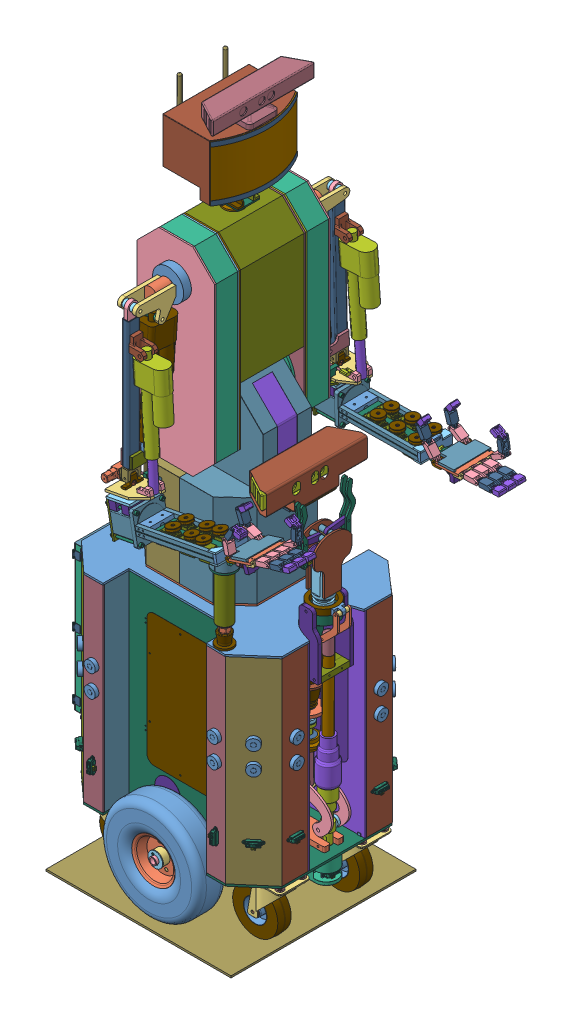
SolidWorks assembly sorbot, configuration По умолчанию. Lengths in mm. (continued)
Mates (geometry in assembly coordinates): (continued)
- Расстояние24: distance = 14 mm anti-aligned: plane of ? through (171.0986 905.6533 109.8374) normal (0.9762 0.216874 0); plane of ? through (184.7654 908.6895 127.5946) normal (-0.9762 -0.216874 0)
- Заблокировать539: lock: unknown of lower.arm.p2-1; unknown of arm.rotate.p9-1
- Заблокировать540: lock: unknown of lower.arm.p2-3; unknown of arm.rotate.p9-1
- Расстояние25: distance = 0.5 mm anti-aligned: plane of lower.arm.p3-1 through (42.4949 859.0482 146.4722) normal (-0.982605 -0.185706 0); plane of arm.rotate-1/SY85STH65-2808A-1 through (42.1893 857.9727 140.2746) normal (0.982605 0.185706 0)
- Заблокировать541: lock: unknown of lower.arm.p2-2; unknown of arm.rotate.p9-2
- Совпадение1112: coincident anti-aligned: plane of lower.arm.p3-1 through (42.4949 859.0482 134.0356) normal (-0.185706 0.982605 0); plane of arm.rotate.p9-1 through (42.4949 859.0482 107.7746) normal (0.185706 -0.982605 0)
- Совпадение1114: coincident anti-aligned: plane of lower.arm.p3-1 through (42.8663 857.083 134.0356) normal (0.185706 -0.982605 0); plane of arm.rotate.p9-2 through (72.3444 862.6542 107.7746) normal (-0.185706 0.982605 0)
- Концентричный603: concentric anti-aligned: cylinder of arm.rotate-1/SY85STH65-2808A-1 through (71.6674 863.5439 140.2746) axis (-0.982605 -0.185706 0) radius 6; cylinder of arm.rotate.p9-1 through (42.6806 858.0656 140.2746) axis (0.982605 0.185706 0) radius 6
- Концентричный604: concentric aligned: cylinder of arm.rotate-1/SY85STH65-2808A-1 through (71.6674 863.5439 140.2746) axis (-0.982605 -0.185706 0) radius 6; cylinder of arm.rotate.p9-2 through (72.1587 863.6368 140.2746) axis (-0.982605 -0.185706 0) radius 6
- Совпадение1115: coincident anti-aligned: plane of lower.arm.p2-1 through (252.7724 898.7894 173.2746) normal (0.982605 0.185706 0); plane of lower.arm.p8-2 through (256.6003 878.5354 183.2746) normal (-0.982605 -0.185706 0)
- Расстояние26: distance = 120 mm aligned: unknown of arm.actuator100mm..p1-1; unknown of arm.actuator100mm.p2-1
- Расстояние27: distance = 30 mm aligned: unknown of arm.actuator100mm..p1-1; unknown of arm.actuator100mm.p2-1
- Совпадение1119: coincident anti-aligned: plane of arm.rotate.p8-1 through (-3.0887 921.1635 130.5417) normal (0.185706 -0.982605 0); plane of arm.rotate.p6-1 through (-41.1593 913.9684 182.7746) normal (-0.185706 0.982605 0)
- Совпадение1120: coincident anti-aligned: plane of arm.rotate.p6-1 through (-46.5956 921.7238 182.7746) normal (0.060639 0.99816 0); plane of arm.rotate.p7-1 through (19.283 917.7216 160.2746) normal (-0.060639 -0.99816 0)
- Заблокировать542: lock: unknown of arm.rotate.p8-1; unknown of arm.rotate.p6-1
- Совпадение1122: coincident aligned: unknown of arm.rotate.p6-1; unknown of arm.rotate.p7-1
- Заблокировать543: lock: unknown of arm.rotate.p6-1; unknown of arm.rotate.p7-1
- Совпадение1123: coincident anti-aligned: plane of arm.rotate.p6-1 through (-46.5956 921.7238 182.7746) normal (0.060639 0.99816 0); plane of arm.rotate.p7-2 through (19.283 917.7216 130.2746) normal (-0.060639 -0.99816 0)
- Касательный40: tangent anti-aligned: plane of arm.rotate.p7-2 through (56.0951 948.6321 130.2746) normal (0 0 1); cylinder of arm.actuator100mm.p2-1 through (49.2564 930.6158 140.2746) axis (-0.061067 0.998134 0) radius 10
- Концентричный606: concentric aligned: cylinder of arm.actuator100mm.p2-1 through (48.7373 939.0999 165.2746) axis (0 0 -1) radius 4; cylinder of arm.rotate.p7-2 through (48.7373 939.0999 130.2746) axis (0 0 -1) radius 4
- Совпадение1124: coincident aligned: plane of arm.rotate.p6-1 through (55.2167 915.5386 97.7746) normal (0.99816 -0.060639 0); plane of arm.rotate.p7-2 through (57.0359 945.4834 120.2746) normal (0.99816 -0.060639 0)
- Заблокировать544: lock: unknown of arm.rotate.p6-1; unknown of arm.rotate.p7-2
- Концентричный607: concentric aligned: cylinder of arm.actuator100mm.p2-1 through (48.7373 939.0999 165.2746) axis (0 0 -1) radius 4; cylinder of arm.rotate.p7-1 through (48.7373 939.0999 160.2746) axis (0 0 -1) radius 4
- Совпадение1125: coincident: unknown of ?; unknown of arm.rotate.p10-1
- Совпадение1126: coincident: unknown of ?; unknown of arm.rotate.p10-1
- Совпадение1127: coincident anti-aligned: unknown of ?; unknown of arm.rotate.p10-1
- Заблокировать545: lock: unknown of ?; unknown of arm.rotate.p10-1
- Расстояние28: distance = 9.5 mm anti-aligned: plane of arm.rotate.p6-1 through (-40.0451 908.0728 182.7746) normal (0.185706 -0.982605 0); plane of arm.rotate.p10-1 through (25.5885 910.8089 182.7746) normal (-0.185706 0.982605 0)
- Касательный41: tangent anti-aligned: unknown of arm.rotate.p10-1; sphere of ?
- Касательный42: tangent anti-aligned: plane of arm.rotate.p10-1 through (25.5885 910.8089 182.7746) normal (-0.185706 0.982605 0); unknown of ?
- Концентричный608: concentric aligned: cylinder of arm.rotate.p10-1 through (-6.3462 904.7735 140.2746) axis (0.185706 -0.982605 0) radius 4; cylinder of ? through (-7.6926 911.8974 140.2746) axis (0.185706 -0.982605 0) radius 18.2
- Концентричный609: concentric anti-aligned: cylinder of arm.rotate.p6-1 through (-8.1104 914.1082 140.2746) axis (-0.185706 0.982605 0) radius 4; cylinder of arm.rotate.p10-1 through (-6.3462 904.7735 140.2746) axis (0.185706 -0.982605 0) radius 4
- Совпадение1128: coincident anti-aligned: plane of arm.rotate.p10-1 through (26.7027 904.9133 182.7746) normal (0.185706 -0.982605 0); plane of bolt.m8.short-1 through (-5.232 898.8778 140.2746) normal (-0.185706 0.982605 0)
- Концентричный610: concentric aligned: cylinder of arm.rotate.p10-1 through (-6.3462 904.7735 140.2746) axis (0.185706 -0.982605 0) radius 4; cylinder of bolt.m8.short-1 through (-11.7317 933.269 140.2746) axis (0.185706 -0.982605 0) radius 4
- Концентричный612: concentric aligned: cylinder of bolt.m8.short-1 through (-13.9627 933.3208 140.2746) axis (-0.157334 -0.987545 0) radius 4; cylinder of m8.nut-1 through (-14.9853 926.9018 140.2746) axis (-0.157334 -0.987545 0) radius 4
- Заблокировать547: lock: unknown of arm.rotate.p6-1; unknown of arm.rotate.p10-1
- Совпадение1129: coincident anti-aligned: plane of arm.rotate.p10-1 through (25.5885 910.8089 182.7746) normal (-0.185706 0.982605 0); plane of arm.elbow.rotate.p3-1 through (-6.3462 904.7735 140.2746) normal (0.185706 -0.982605 0)
- Концентричный613: concentric aligned: cylinder of ? through (-7.6926 911.8974 140.2746) axis (0.185706 -0.982605 0) radius 18.2; cylinder of arm.elbow.rotate.p3-1 through (-8.0176 913.6169 140.2746) axis (0.185706 -0.982605 0) radius 18.2
- Совпадение1130: coincident anti-aligned: plane of arm.rotate.p10-1 through (25.5885 910.8089 182.7746) normal (-0.185706 0.982605 0); plane of arm.elbow.rotate.p4-1 through (-6.3462 904.7735 140.2746) normal (0.185706 -0.982605 0)
- Концентричный614: concentric aligned: cylinder of arm.elbow.rotate.p3-1 through (-8.0176 913.6169 140.2746) axis (0.185706 -0.982605 0) radius 11; cylinder of arm.elbow.rotate.p4-1 through (-7.6461 911.6517 140.2746) axis (0.185706 -0.982605 0) radius 11
- Совпадение1140: coincident anti-aligned: plane of arm.rotate.p6-1 through (-48.1819 925.1023 182.7746) normal (0.157334 0.987545 0); plane of m8.nut-1 through (-12.3806 919.3985 146.7746) normal (-0.157334 -0.987545 0)
- Заблокировать549: lock: unknown of arm.rotate.p6-1; unknown of m8.nut-1
- Заблокировать550: lock: unknown of arm.rotate.p6-1; unknown of arm.rotate.p11-1
- Заблокировать551: lock: unknown of arm.elbow.rotate.p1-1; unknown of arm.rotate.p11-1
- Заблокировать552: lock: unknown of arm.elbow.rotate.p1-1; unknown of arm.elbow.rotate.p5-1
- Заблокировать553: lock: unknown of arm.rotate.p7-2; unknown of arm.elbow.rotate.p6-1
- Параллельность209: parallel aligned: plane of arm.rotate.p9-1 through (40.6378 868.8743 107.7746) normal (-0.185706 0.982605 0); plane of arm.rotate.p10-1 through (25.5885 910.8089 182.7746) normal (-0.185706 0.982605 0)
- Концентричный615: concentric aligned: cylinder of arm.elbow.rotate.p5-1 through (35.8794 941.7075 114.7746) axis (-0.982605 -0.185706 0) radius 2.5; cylinder of arm.elbow.rotate.p11-1 through (8.5139 936.5356 114.7746) axis (-0.982605 -0.185706 0) radius 2.5
- Концентричный616: concentric anti-aligned: cylinder of arm.rotate.p10-1 through (18.8419 903.4277 105.7746) axis (-0.185706 0.982605 0) radius 2.5; cylinder of arm.elbow.rotate.p12-1 through (16.8919 913.745 105.7746) axis (0.185706 -0.982605 0) radius 2.5
- Совпадение1141: coincident anti-aligned: plane of arm.rotate.p10-1 through (25.5885 910.8089 182.7746) normal (-0.185706 0.982605 0); plane of arm.elbow.rotate.p12-1 through (8.8842 907.6519 93.7746) normal (0.185706 -0.982605 0)
- Параллельность207: parallel aligned: plane of arm.rotate.p6-1 through (59.0664 932.9105 182.7746) normal (0 0 1); plane of arm.rotate.p10-1 through (-38.2809 898.738 182.7746) normal (0 0 1)
- Концентричный617: concentric aligned: cylinder of arm.elbow.rotate.p11-1 through (4.2377 932.2373 93.7746) axis (0.185706 -0.982605 0) radius 2.5; cylinder of arm.elbow.rotate.p12-1 through (8.0485 912.0737 93.7746) axis (0.185706 -0.982605 0) radius 2.5
- Концентричный619: concentric anti-aligned: cylinder of arm.elbow.rotate.p5-1 through (35.8794 941.7075 114.7746) axis (-0.982605 -0.185706 0) radius 2.5; cylinder of arm.elbow.rotate.p13-1 through (-38.1599 927.7145 114.7746) axis (0.982605 0.185706 0) radius 2.5
- Совпадение1142: coincident anti-aligned: plane of arm.elbow.rotate.p1-1 through (-37.3429 925.2763 117.1746) normal (0 0 1); plane of arm.elbow.rotate.p13-1 through (-37.6868 925.2113 117.1746) normal (0 0 -1)
- Совпадение1144: coincident anti-aligned: plane of arm.elbow.rotate.p1-1 through (-43.0729 926.786 114.7746) normal (0.982605 0.185706 0); plane of arm.elbow.rotate.p13-1 through (-43.0729 926.786 114.7746) normal (-0.982605 -0.185706 0)
- Концентричный620: concentric anti-aligned: cylinder of arm.elbow.rotate.p13-1 through (-43.0729 926.786 114.7746) axis (0.982605 0.185706 0) radius 4.5; cylinder of arm.elbow.rotate.p14-1 through (-31.773 928.9216 114.7746) axis (-0.982605 -0.185706 0) radius 4.5
- Совпадение1145: coincident anti-aligned: plane of arm.rotate.p11-1 through (-39.1941 914.3398 97.7746) normal (0.982605 0.185706 0); plane of arm.elbow.rotate.p14-1 through (-41.599 927.0645 114.7746) normal (-0.982605 -0.185706 0)
- Параллельность211: parallel aligned: plane of lower.arm.p2-2 through (240.557 838.2014 183.2746) normal (0 0 1); plane of palm.tilt.p1-1 through (42.857 823.2014 151.7746) normal (0 0 1)
- Расстояние30: distance = 31.5 mm aligned: plane of lower.arm.p2-2 through (240.557 838.2014 183.2746) normal (0 0 1); plane of palm.tilt.p1-1 through (42.857 823.2014 151.7746) normal (0 0 1)
- Совпадение1148: coincident anti-aligned: plane of arm.rotate.p9-2 through (56.557 838.2014 172.7746) normal (1 0 0); plane of palm.tilt.p1-1 through (56.557 838.2014 140.4246) normal (-1 0 0)
- Касательный45: tangent anti-aligned: plane of lower.arm.p3-1 through (26.557 848.2014 134.0356) normal (0 -1 0); cylinder of palm.tilt.p1-1 through (70.257 838.2014 140.4246) axis (-1 0 0) radius 10
- Заблокировать556: lock: unknown of arm.rotate.p9-2; unknown of palm.tilt.p1-1
- Заблокировать558: lock: unknown of palm.tilt.p1-1; unknown of palm.drives.fixture-2
- Концентричный624: concentric aligned: cylinder of palm.tilt.p1-1 through (97.1945 857.1737 140.4246) axis (-0.982605 -0.185706 0) radius 1.5; cylinder of palm.lift.p2-2 through (252.4461 886.5153 140.4246) axis (-0.982605 -0.185706 0) radius 2.5
- Совпадение1156: coincident anti-aligned: plane of palm.tilt.p1-1 through (97.1945 857.1737 140.4246) normal (0.982605 0.185706 0); plane of palm.lift.p2-2 through (97.1945 857.1737 140.4246) normal (-0.982605 -0.185706 0)
- Заблокировать559: lock: unknown of palm.drive.thread.fixture.p2-1; unknown of m3x8-1
- Заблокировать560: lock: unknown of palm.drive.thread.fixture.p2-1; unknown of m3x8-2
- Заблокировать561: lock: unknown of palm.lift.p2-2; unknown of palm.drive.thread.fixture.p2-1
- Концентричный625: concentric aligned: cylinder of palm.lift.p2-2 through (252.4461 886.5153 140.4246) axis (-0.982605 -0.185706 0) radius 2.5; cylinder of palm.drive.thread.fixture-1 through (254.516 886.9065 140.4246) axis (-0.982605 -0.185706 0) radius 2.5
- Совпадение1157: coincident anti-aligned: plane of lower.arm.p3-1 through (42.8663 857.083 134.0356) normal (0.185706 -0.982605 0); plane of palm.drive.thread.fixture-1 through (245.7807 895.4326 155.4246) normal (-0.185706 0.982605 0)
- Заблокировать562: lock: unknown of lower.arm.p3-1; unknown of palm.drive.thread.fixture-1
- Заблокировать563: lock: unknown of lower.arm.p8-2; unknown of palm.lift.fixture-1
- Концентричный626: concentric aligned: cylinder of palm.lift.fixture-1 through (273.752 896.6482 125.2746) axis (0 0 1) radius 3; cylinder of palm.lift.fixture.p2-1 through (273.752 896.6482 125.2746) axis (0 0 1) radius 3
- Совпадение1164: coincident anti-aligned: plane of lower.arm.p3-1 through (42.8663 857.083 134.0356) normal (0.185706 -0.982605 0); plane of PALM.LIFT.THREAD.FIXTURE.P3-1 through (121.2398 871.8951 145.2958) normal (-0.185706 0.982605 0)
- Концентричный627: concentric anti-aligned: cylinder of ? through (252.4461 886.5153 140.4246) axis (-0.982605 -0.185706 0) radius 2.5; cylinder of PALM.LIFT.THREAD.FIXTURE.P3-1 through (123.0968 862.0691 140.4246) axis (0.982605 0.185706 0) radius 2.5
- Заблокировать565: lock: unknown of ?; unknown of ?
- Концентричный628: concentric aligned: cylinder of palm.lift.p2-2 through (252.4461 886.5153 140.4246) axis (-0.982605 -0.185706 0) radius 2.5; cylinder of palm.lift.drive.nut-1 through (183.8748 873.5557 140.4246) axis (-0.982605 -0.185706 0) radius 2.5
- Совпадение1167: coincident anti-aligned: plane of lower.arm.p3-1 through (42.8663 857.083 134.0356) normal (0.185706 -0.982605 0); plane of palm.lift.nut.fixture-1 through (169.2438 880.9676 140.4246) normal (-0.185706 0.982605 0)
- Совпадение1168: coincident anti-aligned: plane of palm.lift.drive.nut-1 through (180.9269 872.9986 140.4246) normal (-0.982605 -0.185706 0); plane of palm.lift.nut.fixture-1 through (184.2697 855.3117 150.4246) normal (0.982605 0.185706 0)
- Концентричный629: concentric aligned: cylinder of palm.lift.nut.fixture-2 through (171.1009 871.1415 140.4246) axis (0.982605 0.185706 0) radius 4.5; cylinder of palm.lift.drive.nut-1 through (171.1009 871.1415 140.4246) axis (0.982605 0.185706 0) radius 4.5
- Совпадение1169: coincident anti-aligned: plane of lower.arm.p3-1 through (42.8663 857.083 134.0356) normal (0.185706 -0.982605 0); plane of palm.lift.nut.fixture-2 through (179.0699 882.8247 140.4246) normal (-0.185706 0.982605 0)
- Совпадение1170: coincident anti-aligned: plane of palm.lift.drive.nut-1 through (180.9269 872.9986 140.4246) normal (-0.982605 -0.185706 0); plane of palm.lift.nut.fixture-2 through (184.2697 855.3117 130.4246) normal (0.982605 0.185706 0)
- Концентричный630: concentric aligned: cylinder of palm.lift.p4-1 through (286.5037 879.7822 140.4246) axis (-0.982605 -0.185706 0) radius 2; cylinder of palm.drive.thread.fixture-1 through (256.9192 874.1909 140.4246) axis (-0.982605 -0.185706 0) radius 2
- Заблокировать566: lock: unknown of palm.lift.nut.fixture-1; unknown of palm.lift.p4-1
- Совпадение1173: coincident anti-aligned: plane of palm.lift.fixture-1 through (267.539 889.3678 145.2746) normal (0 0 1); plane of palm.lift.fixture.p2-1 through (259.2428 898.2051 145.2746) normal (0 0 -1)
- Концентричный631: concentric aligned: cylinder of palm.lift.p4-1 through (286.5037 879.7822 140.4246) axis (-0.982605 -0.185706 0) radius 2; cylinder of palm.lift.fixture.p6-1 through (286.5037 879.7822 140.4246) axis (-0.982605 -0.185706 0) radius 2
- Совпадение1174: coincident aligned: plane of palm.lift.p4-1 through (286.5037 879.7822 140.4246) normal (0.982605 0.185706 0); plane of palm.lift.fixture.p6-1 through (286.5037 879.7822 140.4246) normal (0.982605 0.185706 0)
- Совпадение1175: coincident anti-aligned: plane of palm.lift.fixture.p6-1 through (295.2792 887.1977 142.4246) normal (0 0 -1); plane of palm.lift.fixture.p7-1 through (292.1321 880.846 142.4246) normal (0 0 1)
- Концентричный632: concentric anti-aligned: cylinder of palm.lift.fixture.p6-1 through (292.1321 880.846 134.4246) axis (0 0 1) radius 2; cylinder of palm.lift.fixture.p7-1 through (292.1321 880.846 142.4246) axis (0 0 -1) radius 2
- Совпадение1181: coincident anti-aligned: plane of palm.fixture.p14-1 through (318.5768 925.7636 155.9704) normal (-0.311571 0.950223 0); plane of m6.washer-1 through (284.4317 914.5677 140.506) normal (0.311571 -0.950223 0)
- Концентричный634: concentric anti-aligned: cylinder of palm.fixture.p14-1 through (286.3011 908.8663 140.506) axis (-0.311571 0.950223 0) radius 3; cylinder of m6.washer-1 through (283.902 916.183 140.506) axis (0.311571 -0.950223 0) radius 3.25
- Концентричный635: concentric aligned: cylinder of palm.lift.fixture.p2-1 through (291.037 894.4229 140.506) axis (-0.311571 0.950223 0) radius 3; cylinder of m6.washer-2 through (290.0088 897.5587 140.506) axis (-0.311571 0.950223 0) radius 3.25
- Концентричный636: concentric aligned: cylinder of palm.fixture.p14-1 through (286.3011 908.8663 140.506) axis (-0.311571 0.950223 0) radius 3; cylinder of palm.lift.fixture.p2-1 through (291.037 894.4229 140.506) axis (-0.311571 0.950223 0) radius 3
- Совпадение1184: coincident anti-aligned: plane of palm.lift.fixture.p2-1 through (281.0507 896.4104 125.2746) normal (0.311571 -0.950223 0); plane of m6.washer-2 through (289.4791 899.1741 140.506) normal (-0.311571 0.950223 0)
- Концентричный637: concentric anti-aligned: cylinder of palm.lift.fixture.p2-1 through (291.037 894.4229 140.506) axis (-0.311571 0.950223 0) radius 3; cylinder of m6.washer-3 through (286.3011 908.8663 140.506) axis (0.311571 -0.950223 0) radius 3.25
- Совпадение1185: coincident anti-aligned: plane of palm.lift.fixture.p2-1 through (266.9997 900.7485 125.2746) normal (-0.311571 0.950223 0); plane of m6.washer-3 through (286.8308 907.251 140.506) normal (0.311571 -0.950223 0)
- Совпадение1186: coincident anti-aligned: plane of palm.fixture.p14-1 through (320.4462 920.0622 155.9704) normal (0.311571 -0.950223 0); plane of m6.washer-3 through (286.3011 908.8663 140.506) normal (-0.311571 0.950223 0)
- Заблокировать567: lock: unknown of palm.lift.fixture.p2-1; unknown of palm.lift.on-palm.fixture-2
- Концентричный639: concentric aligned: cylinder of palm.lift.fixture.p7-1 through (305.2733 893.1467 142.4246) axis (0 0 -1) radius 2; cylinder of palm.lift.on-palm.fixture-2 through (305.2733 893.1467 153.2746) axis (0 0 -1) radius 2
- Концентричный640: concentric aligned: cylinder of palm.drive.thread.fixture.p2-2 through (326.1771 915.9699 145.3733) axis (-0.012247 -0.004016 0.999917) radius 1.5; cylinder of palm.lift.p1-1 through (326.1091 915.9476 150.9228) axis (-0.012247 -0.004016 0.999917) radius 1.5
- Заблокировать569: lock: unknown of palm.p1-3; unknown of palm.tilit.fixture-1
- Заблокировать570: lock: unknown of palm.lift.p1-1; unknown of palm.tilit.fixture-1
- Совпадение1192: coincident anti-aligned: plane of palm.tilit.p8-1 through (326.1771 915.9699 145.3733) normal (-0.012247 -0.004016 0.999917); plane of palm.drive.thread.fixture.p2-2 through (326.1771 915.9699 145.3733) normal (0.012247 0.004016 -0.999917)
- Концентричный641: concentric anti-aligned: cylinder of palm.drive.thread.fixture.p2-2 through (326.1771 915.9699 145.3733) axis (0.012247 0.004016 -0.999917) radius 2.5; cylinder of palm.tilit.p8-1 through (326.8752 916.1988 88.378) axis (-0.012247 -0.004016 0.999917) radius 2.5
- Совпадение1193: coincident anti-aligned: plane of palm.lift.p1-1 through (325.9934 915.9097 160.372) normal (0.012247 0.004016 -0.999917); plane of palm.drive.thread.fixture.p2-2 through (325.9934 915.9097 160.372) normal (-0.012247 -0.004016 0.999917)
- Совпадение1194: coincident anti-aligned: plane of palm.tilit.p9-1 through (340.8052 933.0521 97.267) normal (-0.311571 0.950223 0); plane of palm.p1-3 through (364.9952 940.9838 91.5947) normal (0.311571 -0.950223 0)
- Совпадение1195: coincident aligned: plane of palm.p1-3 through (291.8649 923.3193 90.628) normal (0.012247 0.004016 -0.999917); plane of palm.tilit.p9-1 through (342.4366 928.3251 91.2675) normal (0.012247 0.004016 -0.999917)
- Совпадение1196: coincident anti-aligned: plane of palm.lift.on-palm.fixture-2 through (305.7565 904.5113 133.5583) normal (0.950223 0.311571 0); plane of palm.tilit.p10-1 through (305.7565 904.5113 153.2746) normal (-0.950223 -0.311571 0)
- Совпадение1197: coincident aligned: plane of palm.lift.on-palm.fixture-2 through (303.1082 912.5882 153.2746) normal (0 0 1); plane of palm.tilit.p10-1 through (317.3615 917.2617 153.2746) normal (0 0 1)
- Совпадение1198: coincident aligned: plane of palm.lift.on-palm.fixture-2 through (305.7565 904.5113 146.9909) normal (0.311571 -0.950223 0); plane of palm.tilit.p10-1 through (320.0099 909.1848 153.2746) normal (0.311571 -0.950223 0)
- Концентричный642: concentric anti-aligned: cylinder of palm.tilit.p8-1 through (326.8752 916.1988 88.378) axis (-0.012247 -0.004016 0.999917) radius 2.5; cylinder of palm.tilit.p11-1 through (326.4209 916.0499 125.4635) axis (0.012247 0.004016 -0.999917) radius 2.5
- Параллельность212: parallel aligned: plane of palm.tilit.p10-1 through (320.0099 909.1848 153.2746) normal (0.311571 -0.950223 0); plane of palm.tilit.p11-1 through (314.9458 908.0777 125.2909) normal (0.311571 -0.950223 0)
- Совпадение1199: coincident anti-aligned: plane of palm.tilit.p10-1 through (320.0099 909.1848 153.2746) normal (0.311571 -0.950223 0); plane of palm.tilit.p12-1 through (316.547 908.0494 140.2746) normal (-0.311571 0.950223 0)
- Концентричный643: concentric anti-aligned: cylinder of palm.tilit.p10-1 through (316.547 908.0494 140.2746) axis (-0.311571 0.950223 0) radius 2; cylinder of palm.tilit.p12-1 through (316.547 908.0494 140.2746) axis (0.311571 -0.950223 0) radius 2
- Заблокировать571: lock: unknown of palm.p1-3; unknown of palm.tilit.p9-1
- Концентричный645: concentric anti-aligned: cylinder of palm.tilit.p11-1 through (317.7835 909.0082 120.329) axis (-0.311571 0.950223 0) radius 2; cylinder of palm.tilit.p12-1 through (317.9473 908.5086 120.329) axis (0.311571 -0.950223 0) radius 2
- Заблокировать572: lock: unknown of palm.drive.thread.fixture-1; unknown of palm.lift.p4-1
- Концентричный646: concentric aligned: cylinder of forearm.rotate.p9-2 through (-12.1948 940.2595 -438.8185) axis (-0.005195 -0.022106 0.999742) radius 2.5; cylinder of arm.rotate.p8-2 through (-12.233 940.097 -431.4713) axis (-0.005195 -0.022106 0.999742) radius 2.5
- Совпадение1200: coincident anti-aligned: plane of forearm.rotate.p9-2 through (-2.569 953.6515 -411.1162) normal (0.005195 0.022106 -0.999742); plane of arm.rotate.p8-2 through (-18.3983 944.5797 -411.3991) normal (-0.005195 -0.022106 0.999742)
- Совпадение1202: coincident anti-aligned: plane of arm.rotate.p6-2 through (-44.3413 918.5492 -379.6011) normal (-0.012385 0.99968 0.022041); plane of arm.rotate.p8-2 through (-5.9858 920.177 -431.8793) normal (0.012385 -0.99968 -0.022041)
- Заблокировать573: lock: unknown of arm.rotate.p6-2; unknown of arm.rotate.p7-3
- Заблокировать574: lock: unknown of arm.rotate.p6-2; unknown of arm.rotate.p7-4
- Концентричный648: concentric anti-aligned: cylinder of arm.rotate.p6-2 through (-11.5491 913.8893 -422.0447) axis (-0.012385 0.99968 0.022041) radius 4; cylinder of bolt.m8.short-2 through (-11.814 935.2675 -421.5734) axis (0.012385 -0.99968 -0.022041) radius 4
- Концентричный649: concentric anti-aligned: cylinder of arm.rotate.p6-2 through (-11.5491 913.8893 -422.0447) axis (-0.012385 0.99968 0.022041) radius 4; cylinder of m8.nut-2 through (-11.7101 926.8852 -421.7582) axis (0.012385 -0.99968 -0.022041) radius 4
- Совпадение1203: coincident anti-aligned: plane of arm.rotate.p6-2 through (-44.3413 918.5492 -379.6011) normal (-0.012385 0.99968 0.022041); plane of m8.nut-2 through (-15.4096 919.6977 -415.4346) normal (0.012385 -0.99968 -0.022041)
- Совпадение1204: coincident anti-aligned: plane of arm.rotate.p8-2 through (-5.812 904.6046 -428.7219) normal (-0.005195 -0.022106 0.999742); plane of m8.nut-2 through (-7.9239 927.0749 -428.236) normal (0.005195 0.022106 -0.999742)
- Концентричный651: concentric aligned: cylinder of forearm.rotate.p12-2 through (-3.3105 975.028 -382.6807) axis (0.999986 0 0.005196) radius 4; cylinder of arm.actuator.p2-5 through (-37.3101 975.028 -382.8574) axis (0.999986 0 0.005196) radius 4
- Заблокировать575: lock: unknown of lower.arm.p2-8; unknown of lower.arm.p3-2
- Заблокировать576: lock: unknown of lower.arm.p2-6; unknown of lower.arm.p3-2
- Заблокировать577: lock: unknown of lower.arm.p3-2; unknown of lower.arm.p8-3
- Заблокировать579: lock: unknown of arm.rotate.p8-2; unknown of m8.nut-2
- Концентричный652: concentric aligned: cylinder of bolt.m8.short-2 through (-11.814 935.2675 -421.5734) axis (0.012385 -0.99968 -0.022041) radius 4; cylinder of arm.elbow.rotate.p4-2 through (-11.512 910.8903 -422.1108) axis (0.012385 -0.99968 -0.022041) radius 4
- Концентричный653: concentric aligned: cylinder of bolt.m8.short-2 through (-11.814 935.2675 -421.5734) axis (0.012385 -0.99968 -0.022041) radius 4; cylinder of ? through (-11.5151 911.1402 -422.1053) axis (0.012385 -0.99968 -0.022041) radius 18.2
- Касательный48: tangent anti-aligned: unknown of ?; plane of arm.rotate.p6-2 through (-44.267 912.5511 -379.7333) normal (0.012385 -0.99968 -0.022041)
- Концентричный655: concentric anti-aligned: cylinder of arm.rotate.p10-2 through (-11.351 897.8945 -422.3973) axis (-0.012385 0.99968 0.022041) radius 4; cylinder of bolt.m8.short-2 through (-11.814 935.2675 -421.5734) axis (0.012385 -0.99968 -0.022041) radius 4
- Касательный50: tangent anti-aligned: unknown of ?; plane of arm.rotate.p10-2 through (21.2926 905.2308 -464.5765) normal (-0.012385 0.99968 0.022041)
- Концентричный656: concentric aligned: cylinder of bolt.m8.short-2 through (-11.814 935.2675 -421.5734) axis (0.012385 -0.99968 -0.022041) radius 4; cylinder of arm.elbow.rotate.p3-2 through (-11.5367 912.8897 -422.0667) axis (0.012385 -0.99968 -0.022041) radius 11
- Совпадение1208: coincident anti-aligned: plane of arm.elbow.rotate.p3-2 through (-11.4253 903.8925 -422.2651) normal (0.012385 -0.99968 -0.022041); plane of arm.rotate.p10-2 through (21.2926 905.2308 -464.5765) normal (-0.012385 0.99968 0.022041)
- Совпадение1215: coincident anti-aligned: plane of arm.rotate.p10-2 through (21.3669 899.2327 -464.7087) normal (0.012385 -0.99968 -0.022041); plane of arm.rotate-2/arm.rotate.p1-3 through (-38.6277 898.4966 -465.0367) normal (-0.012385 0.99968 0.022041)
- Заблокировать582: lock: unknown of arm.rotate.p10-2; unknown of ?
- Концентричный657: concentric aligned: cylinder of arm.actuator100mm.p2-2 through (48.6447 928.0854 -396.9103) axis (0.005195 0.022106 -0.999742) radius 4; cylinder of arm.rotate.p7-3 through (48.824 928.8481 -431.4028) axis (0.005195 0.022106 -0.999742) radius 4
- Концентричный658: concentric aligned: cylinder of arm.rotate-2/SY85STH65-2808A-1 through (58.2497 849.7566 -423.1001) axis (-0.99991 -0.012267 -0.005467) radius 6; cylinder of arm.rotate.p9-3 through (59.2496 849.7688 -423.0946) axis (-0.99991 -0.012267 -0.005467) radius 6
- Концентричный659: concentric anti-aligned: cylinder of arm.rotate-2/SY85STH65-2808A-1 through (58.2497 849.7566 -423.1001) axis (-0.99991 -0.012267 -0.005467) radius 6; cylinder of arm.rotate.p9-4 through (29.2523 849.4008 -423.2587) axis (0.99991 0.012267 0.005467) radius 6
- Параллельность213: parallel anti-aligned: plane of arm.rotate.p9-3 through (59.4308 849.4876 -455.6083) normal (-0.012385 0.99968 0.022041); plane of arm.rotate.p9-4 through (29.4088 851.119 -455.7282) normal (0.012385 -0.99968 -0.022041)
- Совпадение1219: coincident anti-aligned: plane of lower.arm.p3-2 through (29.2723 850.5384 -429.474) normal (-0.012385 0.99968 0.022041); plane of arm.rotate.p9-4 through (29.4088 851.119 -455.7282) normal (0.012385 -0.99968 -0.022041)
- Совпадение1223: coincident aligned: plane of lower.arm.p2-8 through (29.6119 839.3549 -466.49) normal (-0.99991 -0.012267 -0.005467); plane of arm.rotate.p9-3 through (29.2197 837.6859 -391.0095) normal (-0.99991 -0.012267 -0.005467)
- Заблокировать583: lock: unknown of lower.arm.p3-2; unknown of arm.rotate.p9-3
- Расстояние31: distance = 1 mm anti-aligned: plane of arm.rotate.p9-3 through (29.2197 837.6859 -391.0095) normal (-0.99991 -0.012267 -0.005467); plane of arm.rotate-2/SY85STH65-2808A-1 through (28.2524 849.3885 -423.2641) normal (0.99991 0.012267 0.005467)
- Совпадение1224: coincident aligned: plane of arm.rotate.p9-3 through (59.217 838.0539 -390.8455) normal (0.99991 0.012267 0.005467); plane of arm.rotate.p9-4 through (58.9445 860.0469 -390.3606) normal (0.99991 0.012267 0.005467)
- Заблокировать584: lock: unknown of lower.arm.p3-2; unknown of arm.rotate.p9-4
- Заблокировать585: lock: unknown of arm.rotate.p6-2; unknown of arm.rotate.p11.mirr-1
- Совпадение1228: coincident anti-aligned: plane of arm.rotate.p11.mirr-1 through (-44.1127 919.5219 -423.5897) normal (-0.99991 -0.012267 -0.005467); plane of arm.elbow.rotate.p1-2 through (-44.401 942.7787 -423.0475) normal (0.99991 0.012267 0.005467)
- Концентричный660: concentric anti-aligned: cylinder of arm.rotate.p11.mirr-1 through (-44.4134 931.8709 -396.3113) axis (0.99991 0.012267 0.005467) radius 4.5; cylinder of arm.elbow.rotate.p1-2 through (-43.9134 931.877 -396.3085) axis (-0.99991 -0.012267 -0.005467) radius 4.5
- Заблокировать586: lock: unknown of arm.rotate.p11.mirr-1; unknown of arm.elbow.rotate.p1-2
- Совпадение1229: coincident anti-aligned: plane of arm.elbow.rotate.p4-2 through (-11.4253 903.8925 -422.2651) normal (0.012385 -0.99968 -0.022041); plane of arm.rotate.p10-2 through (21.2926 905.2308 -464.5765) normal (-0.012385 0.99968 0.022041)
- Заблокировать587: lock: unknown of arm.rotate.p7-4; unknown of arm.elbow.rotate.p6.mirr-1
- Заблокировать588: lock: unknown of arm.rotate.p11.mirr-1; unknown of arm.elbow.rotate.p13-2
- Концентричный661: concentric anti-aligned: cylinder of arm.elbow.rotate.p13-2 through (-43.5634 931.8813 -396.3066) axis (0.99991 0.012267 0.005467) radius 4.5; cylinder of arm.elbow.rotate.p14-2 through (-32.4144 932.0181 -396.2457) axis (-0.99991 -0.012267 -0.005467) radius 4.5
- Совпадение1230: coincident anti-aligned: plane of arm.rotate.p11.mirr-1 through (-42.1129 919.5464 -423.5788) normal (0.99991 0.012267 0.005467); plane of arm.elbow.rotate.p14-2 through (-42.4135 931.8954 -396.3003) normal (-0.99991 -0.012267 -0.005467)
- Совпадение1231: coincident anti-aligned: plane of arm.elbow.rotate.p1-2 through (-38.5639 931.9427 -396.2793) normal (0.99991 0.012267 0.005467); plane of arm.elbow.rotate.p5-2 through (-38.5639 931.9427 -396.2793) normal (-0.99991 -0.012267 -0.005467)
- Концентричный662: concentric anti-aligned: cylinder of arm.elbow.rotate.p13-2 through (-38.5639 931.9427 -396.2793) axis (0.99991 0.012267 0.005467) radius 2.5; cylinder of arm.elbow.rotate.p5-2 through (36.4293 932.8627 -395.8693) axis (-0.99991 -0.012267 -0.005467) radius 2.5
- Концентричный663: concentric anti-aligned: cylinder of arm.elbow.rotate.p5-2 through (36.4293 932.8627 -395.8693) axis (-0.99991 -0.012267 -0.005467) radius 2.5; cylinder of arm.elbow.rotate.p11-2 through (-1.4172 932.3984 -396.0762) axis (0.99991 0.012267 0.005467) radius 2.5
- Параллельность214: parallel aligned: plane of arm.rotate.p6-2 through (-44.267 912.5511 -379.7333) normal (0.012385 -0.99968 -0.022041); plane of arm.elbow.rotate.p11-2 through (-1.2154 908.6007 -379.597) normal (0.012385 -0.99968 -0.022041)
- Концентричный664: concentric aligned: cylinder of arm.elbow.rotate.p11-2 through (3.5157 928.5672 -375.1299) axis (0.012385 -0.99968 -0.022041) radius 2.5; cylinder of arm.elbow.rotate.p12-2 through (3.7634 908.5736 -375.5707) axis (0.012385 -0.99968 -0.022041) radius 2.5
- Совпадение1232: coincident anti-aligned: plane of arm.elbow.rotate.p11-2 through (-1.2154 908.6007 -379.597) normal (0.012385 -0.99968 -0.022041); plane of arm.elbow.rotate.p12-2 through (3.7634 908.5736 -375.5707) normal (-0.012385 0.99968 0.022041)
- Концентричный665: concentric aligned: cylinder of arm.rotate.p10-2 through (12.8933 903.4304 -387.6401) axis (0.012385 -0.99968 -0.022041) radius 2.5; cylinder of arm.elbow.rotate.p12-2 through (12.8249 908.9493 -387.5184) axis (0.012385 -0.99968 -0.022041) radius 2.5
- Параллельность215: parallel aligned: plane of arm.rotate.p6-2 through (-43.8997 920.4283 -464.5792) normal (-0.99991 -0.012267 -0.005467); plane of arm.rotate.p10-2 through (-43.6272 898.4353 -465.0641) normal (-0.99991 -0.012267 -0.005467)
- Заблокировать589: lock: unknown of arm.rotate.p9-3; unknown of palm.drives.fixture-3
- Заблокировать590: lock: unknown of palm.drives.fixture-3; unknown of palm.tilt.p1-2
- Совпадение1237: coincident anti-aligned: plane of palm.tilt.p1-2 through (73.3338 838.9402 -423.1109) normal (0.99991 0.012267 0.005467); plane of palm.drive.thread.fixture.p2-3 through (73.3338 838.9402 -423.1109) normal (-0.99991 -0.012267 -0.005467)
- Концентричный668: concentric aligned: cylinder of palm.tilt.p1-2 through (82.7829 839.0561 -423.0592) axis (-0.99991 -0.012267 -0.005467) radius 1.5; cylinder of palm.drive.thread.fixture.p2-3 through (88.3324 839.1242 -423.0288) axis (-0.99991 -0.012267 -0.005467) radius 1.5
- Концентричный669: concentric anti-aligned: cylinder of palm.drive.thread.fixture.p2-3 through (88.3324 839.1242 -423.0288) axis (0.99991 0.012267 0.005467) radius 2.5; cylinder of palm.lift.p2-3 through (243.2737 841.0251 -422.1817) axis (-0.99991 -0.012267 -0.005467) radius 2.5
- Концентричный670: concentric aligned: cylinder of palm.lift.p2-3 through (243.2737 841.0251 -422.1817) axis (-0.99991 -0.012267 -0.005467) radius 2.5; cylinder of palm.lift.drive.nut-2 through (168.3752 840.1062 -422.5912) axis (-0.99991 -0.012267 -0.005467) radius 2.5
- Заблокировать591: lock: unknown of palm.drive.thread.fixture.p2-3; unknown of palm.lift.p2-3
- Заблокировать592: lock: unknown of lower.arm.p8-3; unknown of palm.drive.thread.fixture-2
- Концентричный672: concentric anti-aligned: cylinder of palm.lift.drive.nut-2 through (155.3763 839.9467 -422.6623) axis (0.99991 0.012267 0.005467) radius 4.5; cylinder of palm.lift.nut.fixture-3 through (165.3754 840.0694 -422.6076) axis (-0.99991 -0.012267 -0.005467) radius 4.5
- Концентричный673: concentric aligned: cylinder of palm.lift.drive.nut-2 through (155.3763 839.9467 -422.6623) axis (0.99991 0.012267 0.005467) radius 4.5; cylinder of palm.lift.nut.fixture-4 through (155.3763 839.9467 -422.6623) axis (0.99991 0.012267 0.005467) radius 4.5
- Параллельность217: parallel anti-aligned: plane of palm.lift.nut.fixture-4 through (165.2516 850.0662 -422.3872) normal (-0.012385 0.99968 0.022041); plane of lower.arm.p3-2 through (29.2971 848.5391 -429.5181) normal (0.012385 -0.99968 -0.022041)
- Параллельность218: parallel anti-aligned: plane of palm.lift.nut.fixture-3 through (155.2525 849.9435 -422.4419) normal (-0.012385 0.99968 0.022041); plane of lower.arm.p3-2 through (29.2971 848.5391 -429.5181) normal (0.012385 -0.99968 -0.022041)
- Совпадение1239: coincident aligned: plane of palm.lift.nut.fixture-3 through (165.5464 821.8541 -413.0069) normal (0.99991 0.012267 0.005467); plane of palm.lift.nut.fixture-4 through (165.6503 822.2962 -433.0018) normal (0.99991 0.012267 0.005467)
- Совпадение1240: coincident anti-aligned: plane of palm.lift.drive.nut-2 through (165.3754 840.0694 -422.6076) normal (-0.99991 -0.012267 -0.005467); plane of palm.lift.nut.fixture-3 through (165.5464 821.8541 -413.0069) normal (0.99991 0.012267 0.005467)
- Концентричный674: concentric anti-aligned: cylinder of palm.lift.nut.fixture-4 through (155.5366 827.0102 -422.9475) axis (0.99991 0.012267 0.005467) radius 2; cylinder of palm.lift.p4-2 through (270.9675 828.4263 -422.3163) axis (-0.99991 -0.012267 -0.005467) radius 2
- Заблокировать594: lock: unknown of palm.lift.nut.fixture-3; unknown of palm.lift.p4-2
- Заблокировать595: lock: unknown of lower.arm.p8-3; unknown of palm.lift.fixture-2
- Концентричный675: concentric aligned: cylinder of palm.lift.fixture-2 through (263.588 847.6072 -437.0845) axis (-0.005195 -0.022106 0.999742) radius 3; cylinder of palm.lift.fixture.p2-2 through (263.588 847.6072 -437.0845) axis (-0.005195 -0.022106 0.999742) radius 3
- Совпадение1244: coincident anti-aligned: plane of palm.lift.fixture-2 through (256.1542 841.2966 -427.2601) normal (0.005195 0.022106 -0.999742); plane of palm.lift.fixture.p2-2 through (249.8978 852.5761 -427.0432) normal (-0.005195 -0.022106 0.999742)
- Концентричный676: concentric aligned: cylinder of palm.lift.fixture.p2-2 through (279.6623 840.7293 -421.9177) axis (-0.060104 0.997955 0.021755) radius 3; cylinder of m6.washer-4 through (279.464 844.0226 -421.8459) axis (-0.060104 0.997955 0.021755) radius 3.25
- Совпадение1245: coincident anti-aligned: plane of palm.lift.fixture.p2-2 through (270.5872 845.5238 -437.0942) normal (0.060104 -0.997955 -0.021755); plane of m6.washer-4 through (279.3618 845.7191 -421.8089) normal (-0.060104 0.997955 0.021755)
- Концентричный677: concentric anti-aligned: cylinder of palm.lift.fixture.p2-2 through (279.6623 840.7293 -421.9177) axis (-0.060104 0.997955 0.021755) radius 3; cylinder of m6.washer-5 through (278.7488 855.8982 -421.587) axis (0.060104 -0.997955 -0.021755) radius 3.25
- Совпадение1246: coincident anti-aligned: plane of m6.washer-5 through (278.8509 854.2017 -421.624) normal (0.060104 -0.997955 -0.021755); plane of palm.lift.fixture.p2-2 through (258.0981 853.2868 -436.9874) normal (-0.060104 0.997955 0.021755)
- Концентричный678: concentric aligned: cylinder of palm.fixture.p14-2 through (278.7488 855.8982 -421.587) axis (-0.060104 0.997955 0.021755) radius 3; cylinder of palm.lift.fixture.p2-2 through (279.6623 840.7293 -421.9177) axis (-0.060104 0.997955 0.021755) radius 3
- Совпадение1247: coincident anti-aligned: plane of palm.fixture.p14-2 through (314.7351 857.7336 -406.3556) normal (0.060104 -0.997955 -0.021755); plane of m6.washer-5 through (278.7488 855.8982 -421.587) normal (-0.060104 0.997955 0.021755)
- Концентричный680: concentric anti-aligned: cylinder of palm.fixture.p14-2 through (278.7488 855.8982 -421.587) axis (-0.060104 0.997955 0.021755) radius 3; cylinder of m6.washer-6 through (278.286 863.5825 -421.4195) axis (0.060104 -0.997955 -0.021755) radius 3.25
- Совпадение1248: coincident anti-aligned: plane of palm.fixture.p14-2 through (314.3745 863.7213 -406.2251) normal (-0.060104 0.997955 0.021755); plane of m6.washer-6 through (278.3881 861.886 -421.4565) normal (0.060104 -0.997955 -0.021755)
- Совпадение1249: coincident aligned: plane of palm.lift.p4-2 through (270.9675 828.4263 -422.3163) normal (0.99991 0.012267 0.005467); plane of palm.lift.fixture.p6-2 through (270.9675 828.4263 -422.3163) normal (0.99991 0.012267 0.005467)
- Концентричный681: concentric aligned: cylinder of palm.lift.p4-2 through (270.9675 828.4263 -422.3163) axis (-0.99991 -0.012267 -0.005467) radius 2; cylinder of palm.lift.fixture.p6-2 through (270.9675 828.4263 -422.3163) axis (-0.99991 -0.012267 -0.005467) radius 2
- Заблокировать596: lock: unknown of palm.lift.fixture.p2-2; unknown of palm.lift.on-palm.fixture-3
- Концентричный682: concentric anti-aligned: cylinder of palm.lift.on-palm.fixture-3 through (293.0416 835.5977 -409.1898) axis (0.005195 0.022106 -0.999742) radius 2; cylinder of palm.lift.fixture.p7-2 through (293.1196 835.9293 -424.1859) axis (-0.005195 -0.022106 0.999742) radius 2
- Совпадение1250: coincident anti-aligned: plane of palm.lift.fixture.p7-2 through (276.6855 828.4557 -420.4355) normal (-0.005195 -0.022106 0.999742); plane of palm.lift.on-palm.fixture-3 through (297.3768 831.3444 -420.2641) normal (0.005195 0.022106 -0.999742)
- Концентричный683: concentric aligned: cylinder of palm.lift.fixture.p6-2 through (276.7263 828.6292 -428.2835) axis (-0.005195 -0.022106 0.999742) radius 2; cylinder of palm.lift.fixture.p7-2 through (276.7063 828.5441 -424.4345) axis (-0.005195 -0.022106 0.999742) radius 2
- Заблокировать597: lock: unknown of palm.p1-4; unknown of palm.tilit.fixture-2
- Заблокировать598: lock: unknown of palm.tilit.fixture-2; unknown of palm.lift.p1-2
- Концентричный684: concentric aligned: cylinder of palm.drive.thread.fixture.p2-4 through (319.6581 852.5389 -417.0976) axis (-0.005195 -0.022106 0.999742) radius 1.5; cylinder of palm.lift.p1-2 through (319.6293 852.4162 -411.549) axis (-0.005195 -0.022106 0.999742) radius 1.5
- Совпадение1257: coincident anti-aligned: plane of palm.lift.p1-2 through (319.5802 852.2073 -402.1015) normal (0.005195 0.022106 -0.999742); plane of palm.drive.thread.fixture.p2-4 through (319.5802 852.2073 -402.1015) normal (-0.005195 -0.022106 0.999742)
- Совпадение1258: coincident anti-aligned: plane of palm.drive.thread.fixture.p2-4 through (319.6581 852.5389 -417.0976) normal (0.005195 0.022106 -0.999742); plane of palm.tilit.p8-2 through (319.6581 852.5389 -417.0976) normal (-0.005195 -0.022106 0.999742)
- Концентричный685: concentric aligned: cylinder of palm.drive.thread.fixture.p2-4 through (319.6581 852.5389 -417.0976) axis (0.005195 0.022106 -0.999742) radius 2.5; cylinder of palm.tilit.p8-2 through (319.6581 852.5389 -417.0976) axis (0.005195 0.022106 -0.999742) radius 2.5
- Заблокировать599: lock: unknown of palm.p1-4; unknown of palm.tilit.p9-2
- Заблокировать600: lock: unknown of palm.lift.on-palm.fixture-3; unknown of palm.tilit.p10-2
- Совпадение1264: coincident anti-aligned: plane of palm.tilit.p10-2 through (311.367 847.3638 -408.8344) normal (0.060104 -0.997955 -0.021755); plane of palm.tilit.p12-2 through (307.7969 847.4327 -421.8547) normal (-0.060104 0.997955 0.021755)
- Концентричный692: concentric anti-aligned: cylinder of palm.tilit.p10-2 through (307.7969 847.4327 -421.8547) axis (-0.060104 0.997955 0.021755) radius 2; cylinder of palm.tilit.p12-2 through (307.7969 847.4327 -421.8547) axis (0.060104 -0.997955 -0.021755) radius 2
- Концентричный693: concentric aligned: cylinder of palm.tilit.p8-2 through (319.6581 852.5389 -417.0976) axis (0.005195 0.022106 -0.999742) radius 2.5; cylinder of palm.tilit.p11-2 through (319.7594 852.9701 -436.6007) axis (0.005195 0.022106 -0.999742) radius 2.5
- Концентричный695: concentric anti-aligned: cylinder of palm.tilit.p12-2 through (309.6073 847.9757 -441.7652) axis (0.060104 -0.997955 -0.021755) radius 2; cylinder of palm.tilit.p11-2 through (309.5781 848.4611 -441.7546) axis (-0.060104 0.997955 0.021755) radius 2
- Параллельность220: parallel aligned: plane of arm.rotate.p10-2 through (21.2926 905.2308 -464.5765) normal (-0.012385 0.99968 0.022041); plane of arm.rotate.p9-4 through (29.2849 861.1158 -455.5078) normal (-0.012385 0.99968 0.022041)
- Заблокировать601: lock: unknown of palm.lift.p4-2; unknown of palm.drive.thread.fixture-2
- Концентричный696: concentric anti-aligned: cylinder of body.frame.p2-1 through (-12.4903 1112.7235 -136.5542) axis (0 1 0) radius 20; cylinder of SY57STH56-2804A-1 through (-12.4903 1435.8936 -136.5542) axis (0 -1 0) radius 19
- Совпадение1265: coincident anti-aligned: plane of body.frame.p2-1 through (33.4059 1434.2936 -222.3642) normal (0 -1 0); plane of SY57STH56-2804A-1 through (-35.4903 1434.2936 -159.5542) normal (0 1 0)
- Концентричный697: concentric aligned: cylinder of SY57STH56-2804A-1 through (-12.4903 1454.8936 -136.5542) axis (0 -1 0) radius 3.175; cylinder of head.tilt.p1-1 through (-12.4903 1454.7936 -136.5542) axis (0 -1 0) radius 3.175
- Концентричный698: concentric aligned: cylinder of SY57STH56-2804A-1 through (-12.4903 1454.8936 -136.5542) axis (0 -1 0) radius 3.175; cylinder of head.rotate.bearing-1 through (-12.4903 1444.7936 -136.5542) axis (0 -1 0) radius 8.5
- Совпадение1266: coincident anti-aligned: plane of SY57STH56-2804A-1 through (-12.4903 1435.8936 -136.5542) normal (0 1 0); plane of head.rotate.bearing-1 through (-12.4903 1435.8936 -136.5542) normal (0 -1 0)
- Совпадение1267: coincident anti-aligned: plane of SY57STH56-2804A-1 through (-12.4903 1435.8936 -136.5542) normal (0 1 0); plane of head.rotate.bearing.insert-1 through (-12.4903 1435.8936 -136.5542) normal (0 -1 0)
- Концентричный699: concentric aligned: cylinder of SY57STH56-2804A-1 through (-12.4903 1454.8936 -136.5542) axis (0 -1 0) radius 3.175; cylinder of head.rotate.bearing.insert-1 through (-12.4903 1444.3936 -136.5542) axis (0 -1 0) radius 3.175
- Совпадение1268: coincident anti-aligned: plane of head.tilt.p1-1 through (-12.4903 1444.7936 -136.5542) normal (0 -1 0); plane of head.rotate.bearing-1 through (-12.4903 1444.7936 -136.5542) normal (0 1 0)
- Параллельность221: parallel anti-aligned: plane of body.frame.p2-1 through (33.4059 1436.2936 -222.3642) normal (0 1 0); plane of SY42STH47-1 through (-17.6903 1463.2936 -152.0542) normal (0 -1 0)
- Концентричный701: concentric aligned: cylinder of SY42STH47-1 through (-33.8403 1484.4436 -128.0542) axis (0 0 -1) radius 2.5; cylinder of head.tilt.p2-1 through (-33.8403 1484.4436 -134.5542) axis (0 0 -1) radius 2.5
- Заблокировать602: lock: unknown of SY42STH47-1; unknown of head.tilt.p2-1
- Концентричный705: concentric anti-aligned: cylinder of head.tilt.p1-1 through (-2.6766 1437.2936 -156.8012) axis (0 1 0) radius 2; cylinder of head.tilit.p4-1 through (-2.6766 1467.8044 -156.8012) axis (0 -1 0) radius 2
- Концентричный706: concentric anti-aligned: cylinder of head.tilt.p1-1 through (7.7567 1437.2936 -126.7405) axis (0 1 0) radius 2; cylinder of head.tilit.p4-2 through (7.7567 1467.8044 -126.7405) axis (0 -1 0) radius 2
- Концентричный707: concentric anti-aligned: cylinder of head.tilt.p1-1 through (-22.304 1437.2936 -116.3072) axis (0 1 0) radius 2; cylinder of head.tilit.p4-3 through (-22.304 1467.8044 -116.3072) axis (0 -1 0) radius 2
- Концентричный708: concentric anti-aligned: cylinder of head.tilt.p1-1 through (-32.7373 1437.2936 -146.3679) axis (0 1 0) radius 2; cylinder of head.tilit.p4-4 through (-32.7373 1467.8044 -146.3679) axis (0 -1 0) radius 2
- Совпадение1273: coincident anti-aligned: plane of head.tilt.p1-1 through (-12.4903 1441.2936 -136.5542) normal (0 1 0); plane of head.tilit.p4-4 through (-32.7373 1441.2936 -146.3679) normal (0 -1 0)
- Совпадение1274: coincident anti-aligned: plane of head.tilt.p1-1 through (-12.4903 1441.2936 -136.5542) normal (0 1 0); plane of head.tilit.p4-3 through (-22.304 1441.2936 -116.3072) normal (0 -1 0)
- Совпадение1275: coincident anti-aligned: plane of head.tilt.p1-1 through (-12.4903 1441.2936 -136.5542) normal (0 1 0); plane of head.tilit.p4-1 through (-2.6766 1441.2936 -156.8012) normal (0 -1 0)
- Совпадение1276: coincident anti-aligned: plane of head.tilt.p1-1 through (-12.4903 1441.2936 -136.5542) normal (0 1 0); plane of head.tilit.p4-2 through (7.7567 1441.2936 -126.7405) normal (0 -1 0)
- Концентричный709: concentric aligned: cylinder of SY57STH56-2804A-1 through (-12.4903 1454.8936 -136.5542) axis (0 -1 0) radius 3.175; cylinder of head.p1-1 through (-12.4903 1458.2936 -136.5542) axis (0 -1 0) radius 3.175
- Совпадение1277: coincident anti-aligned: plane of head.tilt.p1-1 through (-12.4903 1454.7936 -136.5542) normal (0 1 0); plane of head.p1-1 through (30.0097 1454.7936 -164.0542) normal (0 -1 0)
- Совпадение1278: coincident anti-aligned: plane of head.p1-1 through (30.0097 1458.2936 -164.0542) normal (0 1 0); plane of head.tilit.p5-1 through (30.0097 1458.2936 -148.0542) normal (0 -1 0)
- Совпадение1279: coincident anti-aligned: plane of SY42STH47-1 through (-17.6903 1463.2936 -152.0542) normal (0 -1 0); plane of head.tilit.p5-1 through (30.0097 1463.2936 -152.0542) normal (0 1 0)
